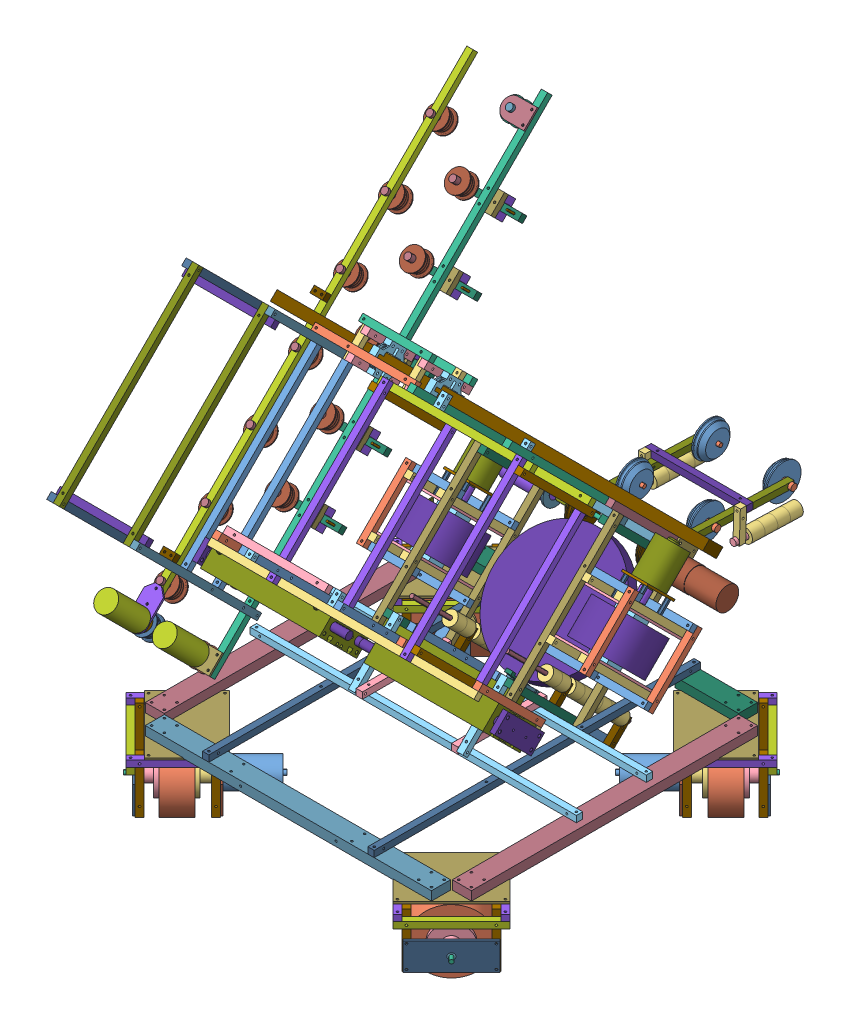
SolidWorks assembly R1, configuration ﾃﾞﾌｫﾙﾄ. Lengths in mm. (continued)
Components (placement in the parent): (continued)
- Copy of Shooter^R1-1: Copy of Shooter^R1 [ﾃﾞﾌｫﾙﾄ] at (-133.6161 -3.3981 632.9203) x (1 0 0) z (0 0.707107 0.707107) size (512.8 479.46 353.57) (virtual, flexible) (continued)
  - Copy of Copy (2) of Copy of Copy of Copy of Copy of Copy (2) of Copy of Copy (2) of 角材１^Copy of Shooter_R1-1: Copy of Copy (2) of Copy of Copy of Copy of Copy of Copy (2) of Copy of Copy (2) of 角材１^Copy of Shooter_R1 [ﾃﾞﾌｫﾙﾄ] at (170 10 140) x (0 0 -1) z (1 0 0) size (250 10 10) (virtual)
  - Part17^Copy of Shooter_R1-2: Part17^Copy of Shooter_R1 [ﾃﾞﾌｫﾙﾄ] at (35 45 -115) x (-0.307741 0.95147 0) z (0 0 1) size (6 6 270) (virtual)
  - Copy (2) of Copy of Copy of Copy of Copy of Copy (2) of Copy of Copy (2) of 角材１^Copy of Shooter_R1-5: Copy (2) of Copy of Copy of Copy of Copy of Copy (2) of Copy of Copy (2) of 角材１^Copy of Shooter_R1 [ﾃﾞﾌｫﾙﾄ] at (30 50 20) x (0 -1 0) z (0 0 1) size (50 10 10) (virtual)
  - Copy of Copy (2) of Copy of Copy of Copy of Copy of Copy (2) of Copy of Copy (2) of 角材１^Copy of Shooter_R1-2: Copy of Copy (2) of Copy of Copy of Copy of Copy of Copy (2) of Copy of Copy (2) of 角材１^Copy of Shooter_R1 [ﾃﾞﾌｫﾙﾄ] at (40 10 140) x (0 0 -1) z (1 0 0) size (250 10 10) (virtual)
  - Copy (3) of Copy of Copy of Copy of Copy of Copy (2) of Copy of Copy (2) of 角材１^Copy of Shooter_R1-1: Copy (3) of Copy of Copy of Copy of Copy of Copy (2) of Copy of Copy (2) of 角材１^Copy of Shooter_R1 [ﾃﾞﾌｫﾙﾄ] at (30 0 -100) size (160 10 10) (virtual)
  - Copy (2) of Copy of Copy of Copy of Copy of Copy (2) of Copy of Copy (2) of 角材１^Copy of Shooter_R1-6: Copy (2) of Copy of Copy of Copy of Copy of Copy (2) of Copy of Copy (2) of 角材１^Copy of Shooter_R1 [ﾃﾞﾌｫﾙﾄ] at (30 50 -110) x (0 -1 0) z (0 0 1) size (50 10 10) (virtual)
  - Copy (2) of Copy of Copy of Copy of Copy of Copy (2) of Copy of Copy (2) of 角材１^Copy of Shooter_R1-7: Copy (2) of Copy of Copy of Copy of Copy of Copy (2) of Copy of Copy (2) of 角材１^Copy of Shooter_R1 [ﾃﾞﾌｫﾙﾄ] at (180 50 -110) x (0 -1 0) z (0 0 1) size (50 10 10) (virtual)
  - Part20^Copy of Shooter_R1-1: Part20^Copy of Shooter_R1 [ﾃﾞﾌｫﾙﾄ] at (185 45 0) x (0 1 0) z (0 0 -1) size (21 21 20) (virtual)
  - Part20^Copy of Shooter_R1-2: Part20^Copy of Shooter_R1 [ﾃﾞﾌｫﾙﾄ] at (185 45 20) x (0 1 0) z (0 0 -1) size (21 21 20) (virtual)
  - Part20^Copy of Shooter_R1-3: Part20^Copy of Shooter_R1 [ﾃﾞﾌｫﾙﾄ] at (185 45 -80) x (0 1 0) z (0 0 -1) size (21 21 20) (virtual)
  - Part20^Copy of Shooter_R1-4: Part20^Copy of Shooter_R1 [ﾃﾞﾌｫﾙﾄ] at (185 45 -20) x (0 1 0) z (0 0 -1) size (21 21 20) (virtual)
  - Part20^Copy of Shooter_R1-5: Part20^Copy of Shooter_R1 [ﾃﾞﾌｫﾙﾄ] at (185 45 -60) x (0 1 0) z (0 0 -1) size (21 21 20) (virtual)
  - Part20^Copy of Shooter_R1-6: Part20^Copy of Shooter_R1 [ﾃﾞﾌｫﾙﾄ] at (185 45 -40) x (0.985931 0.167151 0) z (0 0 -1) size (21 21 20) (virtual)
  - Part20^Copy of Shooter_R1-7: Part20^Copy of Shooter_R1 [ﾃﾞﾌｫﾙﾄ] at (35 45 -20) x (0 1 0) z (0 0 -1) size (21 21 20) (virtual)
  - Part20^Copy of Shooter_R1-8: Part20^Copy of Shooter_R1 [ﾃﾞﾌｫﾙﾄ] at (35 45 20) x (0 1 0) z (0 0 -1) size (21 21 20) (virtual)
  - Part20^Copy of Shooter_R1-9: Part20^Copy of Shooter_R1 [ﾃﾞﾌｫﾙﾄ] at (35 45 -40) x (0 1 0) z (0 0 -1) size (21 21 20) (virtual)
  - Part20^Copy of Shooter_R1-10: Part20^Copy of Shooter_R1 [ﾃﾞﾌｫﾙﾄ] at (35 45 0) x (0 1 0) z (0 0 -1) size (21 21 20) (virtual)
  - Part20^Copy of Shooter_R1-11: Part20^Copy of Shooter_R1 [ﾃﾞﾌｫﾙﾄ] at (35 45 -60) x (0.234145 0.972202 0) z (0 0 -1) size (21 21 20) (virtual)
  - Part20^Copy of Shooter_R1-12: Part20^Copy of Shooter_R1 [ﾃﾞﾌｫﾙﾄ] at (35 45 -80) x (0 1 0) z (0 0 -1) size (21 21 20) (virtual)
  - Part20^Copy of Shooter_R1-21: Part20^Copy of Shooter_R1 [ﾃﾞﾌｫﾙﾄ] at (35 45 70) x (0 1 0) z (0 0 -1) size (21 21 20) (virtual)
  - Part20^Copy of Shooter_R1-22: Part20^Copy of Shooter_R1 [ﾃﾞﾌｫﾙﾄ] at (35 45 50) x (0 1 0) z (0 0 -1) size (21 21 20) (virtual)
  - Part20^Copy of Shooter_R1-23: Part20^Copy of Shooter_R1 [ﾃﾞﾌｫﾙﾄ] at (185 45 70) x (0.413014 0.910725 0) z (0 0 -1) size (21 21 20) (virtual)
  - Part20^Copy of Shooter_R1-24: Part20^Copy of Shooter_R1 [ﾃﾞﾌｫﾙﾄ] at (185 45 50) x (-0.320274 0.947325 0) z (0 0 -1) size (21 21 20) (virtual)
  - Copy of Copy of Copy of Copy (2) of Copy of Copy (2) of Copy of Copy (2) of 角材１^Copy of Shooter_R1-1: Copy of Copy of Copy of Copy (2) of Copy of Copy (2) of Copy of Copy (2) of 角材１^Copy of Shooter_R1 [ﾃﾞﾌｫﾙﾄ] at (190 16.9239 46.0051) x (0 -0.707107 0.707107) z (-1 0 0) size (140 10 10) (virtual)
  - Copy of Copy of Copy of Copy (2) of Copy of Copy (2) of Copy of Copy (2) of 角材１^Copy of Shooter_R1-2: Copy of Copy of Copy of Copy (2) of Copy of Copy (2) of Copy of Copy (2) of 角材１^Copy of Shooter_R1 [ﾃﾞﾌｫﾙﾄ] at (40 16.9239 46.0051) x (0 -0.707107 0.707107) z (-1 0 0) size (140 10 10) (virtual)
  - Copy (2) of Copy of Copy of Copy of Copy (2) of Copy of Copy (2) of 角材１^Copy of Shooter_R1-1: Copy (2) of Copy of Copy of Copy of Copy (2) of Copy of Copy (2) of 角材１^Copy of Shooter_R1 [ﾃﾞﾌｫﾙﾄ] at (190 20 150) x (0 -1 0) z (1 0 0) size (100 10 10) (virtual)
  - Copy (2) of Copy of Copy of Copy of Copy (2) of Copy of Copy (2) of 角材１^Copy of Shooter_R1-2: Copy (2) of Copy of Copy of Copy of Copy (2) of Copy of Copy (2) of 角材１^Copy of Shooter_R1 [ﾃﾞﾌｫﾙﾄ] at (20 20 150) x (0 -1 0) z (1 0 0) size (100 10 10) (virtual)
  - Copy of Part14^Copy of Shooter_R1-1: Copy of Part14^Copy of Shooter_R1 [ﾃﾞﾌｫﾙﾄ] at (45.4135 224.2591 -11.1142) x (0 0.083089 -0.996542) z (0 -0.996542 -0.083089) size (6 150 6) (virtual)
  - Copy of Copy of Copy (2) of Part36^Copy of Shooter_R1-1: Copy of Copy of Copy (2) of Part36^Copy of Shooter_R1 [ﾃﾞﾌｫﾙﾄ] at (36.0361 185.9032 -80.4602) x (0 0.839725 -0.543011) z (-1 0 0) size (16 16 18) (virtual)
  - Copy (2) of Copy of Part33^Copy of Shooter_R1-2: Copy (2) of Copy of Part33^Copy of Shooter_R1 [ﾃﾞﾌｫﾙﾄ] at (-597.1629 304.0265 -20) x (1 0 0) z (0 0 -1) size (90 32 32) (virtual)
  - Copy (2) of Copy (2) of Part36^Copy of Shooter_R1-2: Copy (2) of Copy (2) of Part36^Copy of Shooter_R1 [ﾃﾞﾌｫﾙﾄ] at (159 153.0001 -19.875) x (0 0.001736 0.999998) z (1 0 0) size (22 22 10) (virtual)
  - Copy of Copy of Part36^Copy of Shooter_R1-1: Copy of Copy of Part36^Copy of Shooter_R1 [ﾃﾞﾌｫﾙﾄ] at (180 153.1375 -24.4469) x (0 -0.061762 0.998091) z (1 0 0) size (22 22 10) (virtual)
  - Part22^Copy of Shooter_R1-1: Part22^Copy of Shooter_R1 [ﾃﾞﾌｫﾙﾄ] at (285 218 -20) x (0 0 1) z (0 -1 0) size (37 103 37) (virtual)
  - Part23^Copy of Shooter_R1-1: Part23^Copy of Shooter_R1 [ﾃﾞﾌｫﾙﾄ] at (203 240 -40) x (0 0 1) z (-1 0 0) size (40 52 3) (virtual)
  - Copy of Copy of Copy (2) of Copy of Copy of Copy of Copy of Copy (2) of Copy of Copy (2) of 角材１^Copy of Shooter_R1-1: Copy of Copy of Copy (2) of Copy of Copy of Copy of Copy of Copy (2) of Copy of Copy (2) of 角材１^Copy of Shooter_R1 [ﾃﾞﾌｫﾙﾄ] at (190 240 140) x (0 0 -1) z (1 0 0) size (180 10 10) (virtual)
  - Copy of Copy of Copy (2) of Copy of Copy of Copy of Copy of Copy (2) of Copy of Copy (2) of 角材１^Copy of Shooter_R1-2: Copy of Copy of Copy (2) of Copy of Copy of Copy of Copy of Copy (2) of Copy of Copy (2) of 角材１^Copy of Shooter_R1 [ﾃﾞﾌｫﾙﾄ] at (20 240 140) x (0 0 -1) z (1 0 0) size (180 10 10) (virtual)
  - Part24^Copy of Shooter_R1-1: Part24^Copy of Shooter_R1 [ﾃﾞﾌｫﾙﾄ] at (7 250 -40) x (0 0 1) z (1 0 0) size (40 45 3) (virtual)
  - Copy (4) of Copy of Copy of Copy of Copy of Copy (2) of Copy of Copy (2) of 角材１^Copy of Shooter_R1-2: Copy (4) of Copy of Copy of Copy of Copy of Copy (2) of Copy of Copy (2) of 角材１^Copy of Shooter_R1 [ﾃﾞﾌｫﾙﾄ] at (0 0 10) size (220 10 10) (virtual)
  - Copy (2) of Copy of Copy of Copy of Copy of Copy of Copy of Copy of Copy (2) of Copy of Copy (9) of Copy (2) of 角材１^Copy of Shooter_R1-3: Copy (2) of Copy of Copy of Copy of Copy of Copy of Copy of Copy of Copy (2) of Copy of Copy (9) of Copy (2) of 角材１^Copy of Shooter_R1 [ﾃﾞﾌｫﾙﾄ] at (50 218.3881 -5.6375) x (0 0.683966 -0.729514) z (-1 0 0) size (220 10 10) (virtual)
  - Copy (2) of Copy of Copy of Copy of Copy of Copy of Copy of Copy of Copy (2) of Copy of Copy (9) of Copy (2) of 角材１^Copy of Shooter_R1-4: Copy (2) of Copy of Copy of Copy of Copy of Copy of Copy of Copy of Copy (2) of Copy of Copy (9) of Copy (2) of 角材１^Copy of Shooter_R1 [ﾃﾞﾌｫﾙﾄ] at (180 218.3881 -5.6375) x (0 0.683966 -0.729514) z (-1 0 0) size (220 10 10) (virtual)
  - Copy of Copy of Copy of Copy (2) of Copy of Copy (2) of 角材１^Copy of Shooter_R1-1: Copy of Copy of Copy of Copy (2) of Copy of Copy (2) of 角材１^Copy of Shooter_R1 [ﾃﾞﾌｫﾙﾄ] at (190 324.8583 -104.5774) x (-1 0 0) z (0 -0.683966 0.729514) size (160 10 10) (virtual)
  - Part25^Copy of Shooter_R1-1: Part25^Copy of Shooter_R1 [ﾃﾞﾌｫﾙﾄ] at (170 225 -20) x (1 0 0) z (0 0.001736 0.999998) size (12 54 54) (virtual)
  - Part25^Copy of Shooter_R1-2: Part25^Copy of Shooter_R1 [ﾃﾞﾌｫﾙﾄ] at (50 225 -20) x (-1 0 0) z (0 0.001736 0.999998) size (12 54 54) (virtual)
  - Copy (2) of Copy (2) of Part36^Copy of Shooter_R1-3: Copy (2) of Copy (2) of Part36^Copy of Shooter_R1 [ﾃﾞﾌｫﾙﾄ] at (61 296.9999 -20.125) x (0 0.001736 0.999998) z (-1 0 0) size (22 22 10) (virtual)
  - Copy of Part25^Copy of Shooter_R1-3: Copy of Part25^Copy of Shooter_R1 [ﾃﾞﾌｫﾙﾄ] at (170 361.7931 -165.9028) x (1 0 0) z (0 0.037254 -0.999306) size (14 54 54) (virtual)
  - Part26^Copy of Shooter_R1-3: Part26^Copy of Shooter_R1 [ﾃﾞﾌｫﾙﾄ] at (185 361.7931 -165.9028) x (-1 0 0) z (0 0.008305 -0.999966) size (35 10 10) (virtual)
  - Part26^Copy of Shooter_R1-4: Part26^Copy of Shooter_R1 [ﾃﾞﾌｫﾙﾄ] at (35 361.7931 -165.9028) x (1 0 0) z (0 -0.001736 -0.999998) size (35 10 10) (virtual)
  - Copy of Part25^Copy of Shooter_R1-4: Copy of Part25^Copy of Shooter_R1 [ﾃﾞﾌｫﾙﾄ] at (50 361.7931 -165.9028) x (-1 0 0) z (0 -0.238788 -0.971072) size (14 54 54) (virtual)
  - Copy of Part25^Copy of Shooter_R1-5: Copy of Part25^Copy of Shooter_R1 [ﾃﾞﾌｫﾙﾄ] at (170 279.7173 -78.3611) x (1 0 0) z (0 0.999192 -0.040182) size (14 54 54) (virtual)
  - Part26^Copy of Shooter_R1-5: Part26^Copy of Shooter_R1 [ﾃﾞﾌｫﾙﾄ] at (185 279.7173 -78.3611) x (-1 0 0) z (0 -0.001736 -0.999998) size (35 10 10) (virtual)
  - Part26^Copy of Shooter_R1-6: Part26^Copy of Shooter_R1 [ﾃﾞﾌｫﾙﾄ] at (35 279.7173 -78.3611) x (1 0 0) z (0 -0.001736 -0.999998) size (35 10 10) (virtual)
  - Copy of Part25^Copy of Shooter_R1-6: Copy of Part25^Copy of Shooter_R1 [ﾃﾞﾌｫﾙﾄ] at (50 279.7173 -78.3611) x (-1 0 0) z (0 0.022457 -0.999748) size (14 54 54) (virtual)
  - Copy (3) of Copy of Copy of Copy of Copy (2) of Copy of Copy (2) of 角材１^Copy of Shooter_R1-1: Copy (3) of Copy of Copy of Copy of Copy (2) of Copy of Copy (2) of 角材１^Copy of Shooter_R1 [ﾃﾞﾌｫﾙﾄ] at (190 281.5429 -131.4805) x (0 0.729514 0.683966) z (0 -0.683966 0.729514) size (50 10 10) (virtual)
  - Copy (3) of Copy of Copy of Copy of Copy (2) of Copy of Copy (2) of 角材１^Copy of Shooter_R1-2: Copy (3) of Copy of Copy of Copy of Copy (2) of Copy of Copy (2) of 角材１^Copy of Shooter_R1 [ﾃﾞﾌｫﾙﾄ] at (40 281.5429 -131.4805) x (0 0.729514 0.683966) z (0 -0.683966 0.729514) size (50 10 10) (virtual)
  - Part20^Copy of Shooter_R1-25: Part20^Copy of Shooter_R1 [ﾃﾞﾌｫﾙﾄ] at (185 302.2896 -146.2985) x (0.035115 -0.729064 -0.683544) z (0 -0.683966 0.729514) size (21 21 20) (virtual)
  - Copy of Part26^Copy of Shooter_R1-1: Copy of Part26^Copy of Shooter_R1 [ﾃﾞﾌｫﾙﾄ] at (185 274.931 -117.118) x (0 0.683966 -0.729514) z (-0.990327 0.101225 0.094904) size (105 10 10) (virtual)
  - Part20^Copy of Shooter_R1-26: Part20^Copy of Shooter_R1 [ﾃﾞﾌｫﾙﾄ] at (185 315.9689 -160.8888) x (-0.121292 -0.724128 -0.678916) z (0 -0.683966 0.729514) size (21 21 20) (virtual)
  - Part20^Copy of Shooter_R1-27: Part20^Copy of Shooter_R1 [ﾃﾞﾌｫﾙﾄ] at (185 329.6482 -175.4791) x (0.035115 -0.729064 -0.683544) z (0 -0.683966 0.729514) size (21 21 20) (virtual)
  - Part20^Copy of Shooter_R1-28: Part20^Copy of Shooter_R1 [ﾃﾞﾌｫﾙﾄ] at (185 343.3275 -190.0694) x (0.035115 -0.729064 -0.683544) z (0 -0.683966 0.729514) size (21 21 20) (virtual)
  - Part20^Copy of Shooter_R1-29: Part20^Copy of Shooter_R1 [ﾃﾞﾌｫﾙﾄ] at (35 302.2896 -146.2985) x (0.035115 -0.729064 -0.683544) z (0 -0.683966 0.729514) size (21 21 20) (virtual)
  - Part20^Copy of Shooter_R1-30: Part20^Copy of Shooter_R1 [ﾃﾞﾌｫﾙﾄ] at (35 315.9689 -160.8888) x (-0.121292 -0.724128 -0.678916) z (0 -0.683966 0.729514) size (21 21 20) (virtual)
  - Copy of Part26^Copy of Shooter_R1-2: Copy of Part26^Copy of Shooter_R1 [ﾃﾞﾌｫﾙﾄ] at (35 274.931 -117.118) x (0 0.683966 -0.729514) z (-0.990327 0.101225 0.094904) size (105 10 10) (virtual)
  - Part20^Copy of Shooter_R1-31: Part20^Copy of Shooter_R1 [ﾃﾞﾌｫﾙﾄ] at (35 329.6482 -175.4791) x (0.035115 -0.729064 -0.683544) z (0 -0.683966 0.729514) size (21 21 20) (virtual)
  - Part20^Copy of Shooter_R1-32: Part20^Copy of Shooter_R1 [ﾃﾞﾌｫﾙﾄ] at (35 343.3275 -190.0694) x (0.035115 -0.729064 -0.683544) z (0 -0.683966 0.729514) size (21 21 20) (virtual)
  - Copy of Copy (4) of Copy of Copy of Copy of Copy (2) of Copy of Copy (2) of 角材１^Copy of Shooter_R1-1: Copy of Copy (4) of Copy of Copy of Copy of Copy (2) of Copy of Copy (2) of 角材１^Copy of Shooter_R1 [ﾃﾞﾌｫﾙﾄ] at (366.4 -75 137.9289) x (-1 0 0) z (0 -0.707107 -0.707107) size (512.8 10 10) (virtual)
  - Copy of Copy (4) of Copy of Copy of Copy of Copy (2) of Copy of Copy (2) of 角材１^Copy of Shooter_R1-2: Copy of Copy (4) of Copy of Copy of Copy of Copy (2) of Copy of Copy (2) of 角材１^Copy of Shooter_R1 [ﾃﾞﾌｫﾙﾄ] at (366.4 2.7817 60.1472) x (-1 0 0) z (0 -0.707107 -0.707107) size (512.8 10 10) (virtual)
- Copy of Assem3^R1-1: Copy of Assem3^R1 [ﾃﾞﾌｫﾙﾄ] at (-72.9957 96.2968 385.465) size (686.6 558.76 664.68) (virtual, flexible)
  - Assem5^Copy of Assem3_R1-1: Assem5^Copy of Assem3_R1 [ﾃﾞﾌｫﾙﾄ] at (161.552 -141.335 135.1971) x (1 0 0) z (0 0.000491 1) size (268.6 559.01 664.54) (virtual)
    - Copy of Copy of Copy of Copy of Copy of Copy of Copy of Part4^Assem5_Copy of Assem3_R1-1: Copy of Copy of Copy of Copy of Copy of Copy of Copy of Part4^Assem5_Copy of Assem3_R1 [ﾃﾞﾌｫﾙﾄ] at (-330.1724 90.9576 366.8614) x (1 0 0) z (0 0.70676 0.707454) size (10 750 10) (virtual)
    - Copy of Copy of Copy of Copy of Copy of Copy of Part4^Assem5_Copy of Assem3_R1-1: Copy of Copy of Copy of Copy of Copy of Copy of Part4^Assem5_Copy of Assem3_R1 [ﾃﾞﾌｫﾙﾄ] at (-430.1724 628.6154 -156.1339) x (-1 0 0) z (0 0.70676 0.707454) size (10 720 10) (virtual)
    - Copy of Copy of Copy of Part2^Assem5_Copy of Assem3_R1-1: Copy of Copy of Copy of Part2^Assem5_Copy of Assem3_R1 [ﾃﾞﾌｫﾙﾄ] at (-460.8277 161.547 253.7943) x (-1 0 0) z (0 -0.707454 0.70676) size (20 16 30) (virtual)
    - Copy of Copy of Copy of Copy of Copy of Copy (3) of Part3^Assem5_Copy of Assem3_R1-1: Copy of Copy of Copy of Copy of Copy of Copy (3) of Part3^Assem5_Copy of Assem3_R1 [ﾃﾞﾌｫﾙﾄ] at (-292.1724 156.3418 269.8784) x (0 0.70676 0.707454) z (0.847779 -0.375198 0.37483) size (27 4.5 4.5) (virtual)
    - Copy of Copy (2) of Copy of Copy (4) of Copy of Copy of Copy of Copy (2) of Copy of Copy (2) of 角材１^Assem5_Copy of Assem3_R1-1: Copy of Copy (2) of Copy of Copy (4) of Copy of Copy of Copy of Copy (2) of Copy of Copy (2) of 角材１^Assem5_Copy of Assem3_R1 [ﾃﾞﾌｫﾙﾄ] at (-440.1724 154.6215 317.3952) x (0 0.70676 0.707454) z (-1 0 0) size (260 10 10) (virtual)
    - Copy of Copy of Copy of Copy of Copy (2) of Copy of Copy (2) of Part11^Assem5_Copy of Assem3_R1-2: Copy of Copy of Copy of Copy of Copy (2) of Copy of Copy (2) of Part11^Assem5_Copy of Assem3_R1 [ﾃﾞﾌｫﾙﾄ] at (-435.1724 143.8683 327.8551) x (-0.731652 -0.482256 0.481783) z (-0.681679 0.51761 -0.517102) size (33.4 19.6 33.4) (virtual)
    - Copy of Copy of Copy of Copy of Part2^Assem5_Copy of Assem3_R1-1: Copy of Copy of Copy of Copy of Part2^Assem5_Copy of Assem3_R1 [ﾃﾞﾌｫﾙﾄ] at (-310.1724 182.9266 274.9826) x (1 0 0) z (0 -0.707454 0.70676) size (20 10 30) (virtual)
    - Copy of Copy of Copy of Copy (2) of Copy of Copy of Part5^Assem5_Copy of Assem3_R1-2: Copy of Copy of Copy of Copy (2) of Copy of Copy of Part5^Assem5_Copy of Assem3_R1 [ﾃﾞﾌｫﾙﾄ] at (-418.6839 156.0088 340.0168) x (1 -0.000283 0.000282) z (-0.0004 -0.707454 0.70676) size (10 45 10) (virtual)
    - Copy of Copy of Copy of Copy of Copy (4) of Copy of Copy of Copy of Copy (2) of Copy of Copy (2) of 角材１^Assem5_Copy of Assem3_R1-1: Copy of Copy of Copy of Copy of Copy (4) of Copy of Copy of Copy of Copy (2) of Copy of Copy (2) of 角材１^Assem5_Copy of Assem3_R1 [ﾃﾞﾌｫﾙﾄ] at (-320.1724 154.6284 303.253) x (0 0.70676 0.707454) z (1 0 0) size (270 10 10) (virtual)
    - Copy of Copy of Copy of Copy (3) of Copy of Copy of Copy (2) of Copy of Copy (2) of 角材１^Assem5_Copy of Assem3_R1-2: Copy of Copy of Copy of Copy (3) of Copy of Copy of Copy (2) of Copy of Copy (2) of 角材１^Assem5_Copy of Assem3_R1 [ﾃﾞﾌｫﾙﾄ] at (-282.1724 168.3602 274.8341) x (-1 0 0) z (0 -0.707454 0.70676) size (90 10 10) (virtual)
    - Copy of Copy of Copy of Copy of Copy (2) of Copy of Copy (2) of Part11^Assem5_Copy of Assem3_R1-17: Copy of Copy of Copy of Copy of Copy (2) of Copy of Copy (2) of Part11^Assem5_Copy of Assem3_R1 [ﾃﾞﾌｫﾙﾄ] at (-367.1724 164.823 278.3679) x (0.172855 -0.696805 0.696121) z (0.984947 0.122287 -0.122167) size (33.4 19.6 33.4) (virtual)
    - Copy of Copy of Copy of Copy (2) of Copy of Copy of Part5^Assem5_Copy of Assem3_R1-17: Copy of Copy of Copy of Copy (2) of Copy of Copy of Part5^Assem5_Copy of Assem3_R1 [ﾃﾞﾌｫﾙﾄ] at (-350.7089 153.4616 265.7105) x (0.998482 0.038963 -0.038925) z (-0.055075 0.70638 -0.705687) size (10 45 10) (virtual)
    - Copy of Copy of Copy of Copy (2) of Copy of Copy of Copy (2) of Copy of Copy (2) of 角材１^Assem5_Copy of Assem3_R1-1: Copy of Copy of Copy of Copy (2) of Copy of Copy of Copy (2) of Copy of Copy (2) of 角材１^Assem5_Copy of Assem3_R1 [ﾃﾞﾌｫﾙﾄ] at (-320.1724 550.622 275.1631) x (0 -0.707454 0.70676) z (-1 0 0) size (310 10 10) (virtual)
    - Copy of Copy (2) of Copy of Copy of Copy of Copy (2) of Copy of Copy (2) of 角材１^Assem5_Copy of Assem3_R1-1: Copy of Copy (2) of Copy of Copy of Copy of Copy (2) of Copy of Copy (2) of 角材１^Assem5_Copy of Assem3_R1 [ﾃﾞﾌｫﾙﾄ] at (-310.1724 338.3859 487.191) x (-1 0 0) z (0 -0.70676 -0.707454) size (140 10 10) (virtual)
    - Copy of Copy of Copy of Copy (2) of Copy of Copy of Copy (2) of Copy of Copy (2) of 角材１^Assem5_Copy of Assem3_R1-2: Copy of Copy of Copy of Copy (2) of Copy of Copy of Copy (2) of Copy of Copy (2) of 角材１^Assem5_Copy of Assem3_R1 [ﾃﾞﾌｫﾙﾄ] at (-430.1724 550.622 275.1631) x (0 -0.707454 0.70676) z (-1 0 0) size (310 10 10) (virtual)
    - Copy of Copy of Copy of Copy of Copy of Copy of Copy of Copy of Copy of 角材１^Assem5_Copy of Assem3_R1-1: Copy of Copy of Copy of Copy of Copy of Copy of Copy of Copy of Copy of 角材１^Assem5_Copy of Assem3_R1 [ﾃﾞﾌｫﾙﾄ] at (-430.1724 175.8381 310.3345) x (-1 0 0) z (0 0.70676 0.707454) size (20 10 10) (virtual)
    - Copy of Copy of Copy of Copy of Copy (2) of Copy of Copy of Copy (2) of Copy of Copy (2) of 角材１^Assem5_Copy of Assem3_R1-1: Copy of Copy of Copy of Copy of Copy (2) of Copy of Copy of Copy (2) of Copy of Copy (2) of 角材１^Assem5_Copy of Assem3_R1 [ﾃﾞﾌｫﾙﾄ] at (-350.1724 395.1418 105.3811) x (0 -0.707454 0.70676) z (-1 0 0) size (320 10 10) (virtual)
    - Copy of Copy (2) of Copy of Copy (4) of Copy of Copy of Copy of Copy (2) of Copy of Copy (2) of 角材１^Assem5_Copy of Assem3_R1-2: Copy of Copy (2) of Copy of Copy (4) of Copy of Copy of Copy of Copy (2) of Copy of Copy (2) of 角材１^Assem5_Copy of Assem3_R1 [ﾃﾞﾌｫﾙﾄ] at (-440.1724 366.8576 105.3672) x (0 0.70676 0.707454) z (-1 0 0) size (260 10 10) (virtual)
    - Copy of Copy (2) of Copy of Copy of Copy of Copy (2) of Copy of Copy (2) of 角材１^Assem5_Copy of Assem3_R1-2: Copy of Copy (2) of Copy of Copy of Copy of Copy (2) of Copy of Copy (2) of 角材１^Assem5_Copy of Assem3_R1 [ﾃﾞﾌｫﾙﾄ] at (-310.1724 536.473 289.2982) x (-1 0 0) z (0 -0.70676 -0.707454) size (140 10 10) (virtual)
    - Copy of Copy of Copy of Copy of Copy (4) of Copy of Copy of Copy of Copy (2) of Copy of Copy (2) of 角材１^Assem5_Copy of Assem3_R1-2: Copy of Copy of Copy of Copy of Copy (4) of Copy of Copy of Copy of Copy (2) of Copy of Copy (2) of 角材１^Assem5_Copy of Assem3_R1 [ﾃﾞﾌｫﾙﾄ] at (-320.1724 366.8645 91.2251) x (0 0.70676 0.707454) z (1 0 0) size (270 10 10) (virtual)
    - Copy of Copy of Copy of Copy of Copy (4) of Copy of Copy of Copy (2) of Copy of Copy (2) of 角材１^Assem5_Copy of Assem3_R1-1: Copy of Copy of Copy of Copy of Copy (4) of Copy of Copy of Copy (2) of Copy of Copy (2) of 角材１^Assem5_Copy of Assem3_R1 [ﾃﾞﾌｫﾙﾄ] at (-200.1724 388.0742 98.3066) x (-1 0 0) z (0 0.70676 0.707454) size (160 10 10) (virtual)
    - Copy of Copy of Copy of Copy of Copy of Copy (2) of Copy of Copy of Copy of Copy (2) of Copy of Copy (2) of 角材１^Assem5_Copy of Assem3_R1-1: Copy of Copy of Copy of Copy of Copy of Copy (2) of Copy of Copy of Copy of Copy (2) of Copy of Copy (2) of 角材１^Assem5_Copy of Assem3_R1 [ﾃﾞﾌｫﾙﾄ] at (-310.1724 380.9928 119.5163) x (0 0.707454 -0.70676) z (1 0 0) size (55 10 10) (virtual)
    - Copy of Copy of Copy of Copy (2) of Copy of Copy of Copy of Copy (2) of Copy of Copy (2) of 角材１^Assem5_Copy of Assem3_R1-1: Copy of Copy of Copy of Copy (2) of Copy of Copy of Copy of Copy (2) of Copy of Copy (2) of 角材１^Assem5_Copy of Assem3_R1 [ﾃﾞﾌｫﾙﾄ] at (-290.1724 476.4365 151.3829) x (0 -0.70676 -0.707454) z (-1 0 0) size (100 10 10) (virtual)
    - Copy of Copy of Copy of Copy of Copy of Copy of NHK_r1_guide.STL^Assem5_Copy of Assem3_R1-1: Copy of Copy of Copy of Copy of Copy of Copy of NHK_r1_guide.STL^Assem5_Copy of Assem3_R1 [ﾃﾞﾌｫﾙﾄ] at (-280.1724 419.8958 94.7867) x (0 -0.707454 0.70676) z (-1 0 0) size (45 60 10) (virtual)
    - Copy of Copy of Copy of Copy (4) of Copy of Copy of Copy (2) of Copy of Copy (2) of 角材１^Assem5_Copy of Assem3_R1-1: Copy of Copy of Copy of Copy (4) of Copy of Copy of Copy (2) of Copy of Copy (2) of 角材１^Assem5_Copy of Assem3_R1 [ﾃﾞﾌｫﾙﾄ] at (-200.1724 476.4435 137.2408) x (-1 0 0) z (0 0.70676 0.707454) size (110 10 10) (virtual)
    - Copy of Copy of Copy of Copy (2) of Copy of Copy of Copy of Copy (2) of Copy of Copy (2) of 角材１^Assem5_Copy of Assem3_R1-2: Copy of Copy of Copy of Copy (2) of Copy of Copy of Copy of Copy (2) of Copy of Copy (2) of 角材１^Assem5_Copy of Assem3_R1 [ﾃﾞﾌｫﾙﾄ] at (-290.1724 451.6757 176.1195) x (0 -0.70676 -0.707454) z (-1 0 0) size (100 10 10) (virtual)
    - Copy of Copy of Copy of Copy of Copy of Copy (2) of Copy of Copy of Copy of Copy (2) of Copy of Copy (2) of 角材１^Assem5_Copy of Assem3_R1-2: Copy of Copy of Copy of Copy of Copy of Copy (2) of Copy of Copy of Copy of Copy (2) of Copy of Copy (2) of 角材１^Assem5_Copy of Assem3_R1 [ﾃﾞﾌｫﾙﾄ] at (-310.1724 430.4659 169.0381) x (0 0.707454 -0.70676) z (1 0 0) size (55 10 10) (virtual)
    - Copy of Copy of Copy of Copy of Copy (4) of Copy of Copy of Copy (2) of Copy of Copy (2) of 角材１^Assem5_Copy of Assem3_R1-2: Copy of Copy of Copy of Copy of Copy (4) of Copy of Copy of Copy (2) of Copy of Copy (2) of 角材１^Assem5_Copy of Assem3_R1 [ﾃﾞﾌｫﾙﾄ] at (-200.1724 451.6826 161.9774) x (-1 0 0) z (0 0.70676 0.707454) size (160 10 10) (virtual)
    - Copy of Copy of Copy of Copy of Copy of Copy (2) of Copy of Copy of Copy of Copy (2) of Copy of Copy (2) of 角材１^Assem5_Copy of Assem3_R1-3: Copy of Copy of Copy of Copy of Copy of Copy (2) of Copy of Copy of Copy of Copy (2) of Copy of Copy (2) of 角材１^Assem5_Copy of Assem3_R1 [ﾃﾞﾌｫﾙﾄ] at (-220.1724 430.4659 169.0381) x (0 0.707454 -0.70676) z (1 0 0) size (55 10 10) (virtual)
    - Copy of Copy of Copy of Copy (2) of Copy of Copy of Copy of Copy (2) of Copy of Copy (2) of 角材１^Assem5_Copy of Assem3_R1-3: Copy of Copy of Copy of Copy (2) of Copy of Copy of Copy of Copy (2) of Copy of Copy (2) of 角材１^Assem5_Copy of Assem3_R1 [ﾃﾞﾌｫﾙﾄ] at (-200.1724 451.6757 176.1195) x (0 -0.70676 -0.707454) z (-1 0 0) size (100 10 10) (virtual)
    - Copy of Copy of Copy of Copy (4) of Copy of Copy of Copy (2) of Copy of Copy (2) of 角材１^Assem5_Copy of Assem3_R1-2: Copy of Copy of Copy of Copy (4) of Copy of Copy of Copy (2) of Copy of Copy (2) of 角材１^Assem5_Copy of Assem3_R1 [ﾃﾞﾌｫﾙﾄ] at (-200.1724 412.8351 73.57) x (-1 0 0) z (0 0.70676 0.707454) size (110 10 10) (virtual)
    - Copy of Copy of Copy of Copy of Copy of Copy (2) of Copy of Copy of Copy of Copy (2) of Copy of Copy (2) of 角材１^Assem5_Copy of Assem3_R1-4: Copy of Copy of Copy of Copy of Copy of Copy (2) of Copy of Copy of Copy of Copy (2) of Copy of Copy (2) of 角材１^Assem5_Copy of Assem3_R1 [ﾃﾞﾌｫﾙﾄ] at (-220.1724 380.9928 119.5163) x (0 0.707454 -0.70676) z (1 0 0) size (55 10 10) (virtual)
    - Copy of Copy of Copy of Copy (2) of Copy of Copy of Copy of Copy (2) of Copy of Copy (2) of 角材１^Assem5_Copy of Assem3_R1-4: Copy of Copy of Copy of Copy (2) of Copy of Copy of Copy of Copy (2) of Copy of Copy (2) of 角材１^Assem5_Copy of Assem3_R1 [ﾃﾞﾌｫﾙﾄ] at (-200.1724 476.4365 151.3829) x (0 -0.70676 -0.707454) z (-1 0 0) size (100 10 10) (virtual)
    - Copy of Copy of Copy of Copy of Copy of Copy of NHK_r1_guide.STL^Assem5_Copy of Assem3_R1-2: Copy of Copy of Copy of Copy of Copy of Copy of NHK_r1_guide.STL^Assem5_Copy of Assem3_R1 [ﾃﾞﾌｫﾙﾄ] at (-190.1724 419.8958 94.7867) x (0 -0.707454 0.70676) z (-1 0 0) size (45 60 10) (virtual)
    - Copy of Copy of Copy of Copy of Copy of Copy of Copy of Copy of Copy of 角材１^Assem5_Copy of Assem3_R1-3: Copy of Copy of Copy of Copy of Copy of Copy of Copy of Copy of Copy of 角材１^Assem5_Copy of Assem3_R1 [ﾃﾞﾌｫﾙﾄ] at (-430.1724 412.8351 73.57) x (-1 0 0) z (0 0.70676 0.707454) size (20 10 10) (virtual)
    - Copy of Copy of Copy of roller_R1^Assem5_Copy of Assem3_R1-1: Copy of Copy of Copy of roller_R1^Assem5_Copy of Assem3_R1 [ﾃﾞﾌｫﾙﾄ] at (53.8339 52.095 142.792) x (0.212331 0 0.977198) z (0 1 0) (virtual)
    - Copy of Copy of Copy of Copy of Copy (2) of Copy of Copy of Copy (2) of Copy of Copy (2) of 角材１^Assem5_Copy of Assem3_R1-2: Copy of Copy of Copy of Copy of Copy (2) of Copy of Copy of Copy (2) of Copy of Copy (2) of 角材１^Assem5_Copy of Assem3_R1 [ﾃﾞﾌｫﾙﾄ] at (-350.1724 444.615 154.9029) x (0 -0.707454 0.70676) z (-1 0 0) size (320 10 10) (virtual)
    - Copy of Copy of Copy of Copy (2) of Copy of Copy of Part5^Assem5_Copy of Assem3_R1-5: Copy of Copy of Copy of Copy (2) of Copy of Copy of Part5^Assem5_Copy of Assem3_R1 [ﾃﾞﾌｫﾙﾄ] at (-418.6839 297.4995 198.6648) x (1 -0.000283 0.000282) z (-0.0004 -0.707454 0.70676) size (10 45 10) (virtual)
    - Copy of Copy of Copy of Copy (2) of Copy of Copy of Part5^Assem5_Copy of Assem3_R1-6: Copy of Copy of Copy of Copy (2) of Copy of Copy of Part5^Assem5_Copy of Assem3_R1 [ﾃﾞﾌｫﾙﾄ] at (-418.6839 368.2449 127.9889) x (1 -0.000283 0.000282) z (-0.0004 -0.707454 0.70676) size (10 45 10) (virtual)
    - Copy of Copy of Copy of Copy (2) of Copy of Copy of Part5^Assem5_Copy of Assem3_R1-7: Copy of Copy of Copy of Copy (2) of Copy of Copy of Part5^Assem5_Copy of Assem3_R1 [ﾃﾞﾌｫﾙﾄ] at (-418.6839 438.9903 57.3129) x (1 -0.000283 0.000282) z (-0.0004 -0.707454 0.70676) size (10 45 10) (virtual)
    - Copy of Copy of Copy of Copy (2) of Copy of Copy of Part5^Assem5_Copy of Assem3_R1-8: Copy of Copy of Copy of Copy (2) of Copy of Copy of Part5^Assem5_Copy of Assem3_R1 [ﾃﾞﾌｫﾙﾄ] at (-418.6839 509.7356 -13.3631) x (1 -0.000283 0.000282) z (-0.0004 -0.707454 0.70676) size (10 45 10) (virtual)
    - Copy of Copy of Copy of Copy of Copy (2) of Copy of Copy (2) of Part11^Assem5_Copy of Assem3_R1-5: Copy of Copy of Copy of Copy of Copy (2) of Copy of Copy (2) of Part11^Assem5_Copy of Assem3_R1 [ﾃﾞﾌｫﾙﾄ] at (-435.1724 285.359 186.5031) x (-0.731652 -0.482256 0.481783) z (-0.681679 0.51761 -0.517102) size (33.4 19.6 33.4) (virtual)
    - Copy of Copy of Copy of Copy of Copy (2) of Copy of Copy (2) of Part11^Assem5_Copy of Assem3_R1-6: Copy of Copy of Copy of Copy of Copy (2) of Copy of Copy (2) of Part11^Assem5_Copy of Assem3_R1 [ﾃﾞﾌｫﾙﾄ] at (-435.1724 356.1044 115.8271) x (-0.731652 -0.482256 0.481783) z (-0.681679 0.51761 -0.517102) size (33.4 19.6 33.4) (virtual)
    - Copy of Copy of Copy of Copy of Copy (2) of Copy of Copy (2) of Part11^Assem5_Copy of Assem3_R1-7: Copy of Copy of Copy of Copy of Copy (2) of Copy of Copy (2) of Part11^Assem5_Copy of Assem3_R1 [ﾃﾞﾌｫﾙﾄ] at (-435.1724 426.8498 45.1512) x (-0.731652 -0.482256 0.481783) z (-0.681679 0.51761 -0.517102) size (33.4 19.6 33.4) (virtual)
    - Copy of Copy of Copy of Copy of Copy (2) of Copy of Copy (2) of Part11^Assem5_Copy of Assem3_R1-8: Copy of Copy of Copy of Copy of Copy (2) of Copy of Copy (2) of Part11^Assem5_Copy of Assem3_R1 [ﾃﾞﾌｫﾙﾄ] at (-435.1724 497.5951 -25.5248) x (-0.731652 -0.482256 0.481783) z (-0.681679 0.51761 -0.517102) size (33.4 19.6 33.4) (virtual)
    - Copy of Copy of Copy of Copy (2) of Copy of Copy of Part5^Assem5_Copy of Assem3_R1-18: Copy of Copy of Copy of Copy (2) of Copy of Copy of Part5^Assem5_Copy of Assem3_R1 [ﾃﾞﾌｫﾙﾄ] at (-350.7089 224.207 195.0345) x (0.998482 0.038963 -0.038925) z (-0.055075 0.70638 -0.705687) size (10 45 10) (virtual)
    - Copy of Copy of Copy of Copy (2) of Copy of Copy of Part5^Assem5_Copy of Assem3_R1-19: Copy of Copy of Copy of Copy (2) of Copy of Copy of Part5^Assem5_Copy of Assem3_R1 [ﾃﾞﾌｫﾙﾄ] at (-350.7089 294.9523 124.3585) x (0.998482 0.038963 -0.038925) z (-0.055075 0.70638 -0.705687) size (10 45 10) (virtual)
    - Copy of Copy of Copy of Copy (2) of Copy of Copy of Part5^Assem5_Copy of Assem3_R1-20: Copy of Copy of Copy of Copy (2) of Copy of Copy of Part5^Assem5_Copy of Assem3_R1 [ﾃﾞﾌｫﾙﾄ] at (-350.7089 365.6977 53.6825) x (0.998482 0.038963 -0.038925) z (-0.055075 0.70638 -0.705687) size (10 45 10) (virtual)
    - Copy of Copy of Copy of Copy (2) of Copy of Copy of Part5^Assem5_Copy of Assem3_R1-21: Copy of Copy of Copy of Copy (2) of Copy of Copy of Part5^Assem5_Copy of Assem3_R1 [ﾃﾞﾌｫﾙﾄ] at (-350.7089 436.4431 -16.9934) x (0.998482 0.038963 -0.038925) z (-0.055075 0.70638 -0.705687) size (10 45 10) (virtual)
    - Copy of Copy of Copy of Copy (2) of Copy of Copy of Part5^Assem5_Copy of Assem3_R1-22: Copy of Copy of Copy of Copy (2) of Copy of Copy of Part5^Assem5_Copy of Assem3_R1 [ﾃﾞﾌｫﾙﾄ] at (-350.7089 507.1884 -87.6694) x (0.998482 0.038963 -0.038925) z (-0.055075 0.70638 -0.705687) size (10 45 10) (virtual)
    - Copy of Copy of Copy of Copy of Copy (2) of Copy of Copy (2) of Part11^Assem5_Copy of Assem3_R1-18: Copy of Copy of Copy of Copy of Copy (2) of Copy of Copy (2) of Part11^Assem5_Copy of Assem3_R1 [ﾃﾞﾌｫﾙﾄ] at (-367.1724 235.5683 207.6919) x (0.172855 -0.696805 0.696121) z (0.984947 0.122287 -0.122167) size (33.4 19.6 33.4) (virtual)
    - Copy of Copy of Copy of Copy of Copy (2) of Copy of Copy (2) of Part11^Assem5_Copy of Assem3_R1-19: Copy of Copy of Copy of Copy of Copy (2) of Copy of Copy (2) of Part11^Assem5_Copy of Assem3_R1 [ﾃﾞﾌｫﾙﾄ] at (-367.1724 306.3137 137.0159) x (0.172855 -0.696805 0.696121) z (0.984947 0.122287 -0.122167) size (33.4 19.6 33.4) (virtual)
    - Copy of Copy of Copy of Copy of Copy (2) of Copy of Copy (2) of Part11^Assem5_Copy of Assem3_R1-20: Copy of Copy of Copy of Copy of Copy (2) of Copy of Copy (2) of Part11^Assem5_Copy of Assem3_R1 [ﾃﾞﾌｫﾙﾄ] at (-367.1724 377.0591 66.3399) x (0.172855 -0.696805 0.696121) z (0.984947 0.122287 -0.122167) size (33.4 19.6 33.4) (virtual)
    - Copy of Copy of Copy of Copy of Copy (2) of Copy of Copy (2) of Part11^Assem5_Copy of Assem3_R1-21: Copy of Copy of Copy of Copy of Copy (2) of Copy of Copy (2) of Part11^Assem5_Copy of Assem3_R1 [ﾃﾞﾌｫﾙﾄ] at (-367.1724 447.8044 -4.336) x (0.172855 -0.696805 0.696121) z (0.984947 0.122287 -0.122167) size (33.4 19.6 33.4) (virtual)
    - Copy of Copy of Copy of Copy of Copy (2) of Copy of Copy (2) of Part11^Assem5_Copy of Assem3_R1-22: Copy of Copy of Copy of Copy of Copy (2) of Copy of Copy (2) of Part11^Assem5_Copy of Assem3_R1 [ﾃﾞﾌｫﾙﾄ] at (-367.1724 518.5498 -75.012) x (0.172855 -0.696805 0.696121) z (0.984947 0.122287 -0.122167) size (33.4 19.6 33.4) (virtual)
    - Copy of Copy of Copy of Copy of Part2^Assem5_Copy of Assem3_R1-2: Copy of Copy of Copy of Copy of Part2^Assem5_Copy of Assem3_R1 [ﾃﾞﾌｫﾙﾄ] at (-310.1724 253.6719 204.3067) x (1 0 0) z (0 -0.707454 0.70676) size (20 10 30) (virtual)
    - Copy of Copy of Copy of Copy of Part2^Assem5_Copy of Assem3_R1-3: Copy of Copy of Copy of Copy of Part2^Assem5_Copy of Assem3_R1 [ﾃﾞﾌｫﾙﾄ] at (-310.1724 324.4173 133.6307) x (1 0 0) z (0 -0.707454 0.70676) size (20 10 30) (virtual)
    - Copy of Copy of Copy of Copy of Part2^Assem5_Copy of Assem3_R1-4: Copy of Copy of Copy of Copy of Part2^Assem5_Copy of Assem3_R1 [ﾃﾞﾌｫﾙﾄ] at (-310.1724 395.1626 62.9547) x (1 0 0) z (0 -0.707454 0.70676) size (20 10 30) (virtual)
    - Copy of Copy of Copy of Copy of Part2^Assem5_Copy of Assem3_R1-5: Copy of Copy of Copy of Copy of Part2^Assem5_Copy of Assem3_R1 [ﾃﾞﾌｫﾙﾄ] at (-310.1724 465.908 -7.7213) x (1 0 0) z (0 -0.707454 0.70676) size (20 10 30) (virtual)
    - Copy of Copy of Copy of Copy of Part2^Assem5_Copy of Assem3_R1-6: Copy of Copy of Copy of Copy of Part2^Assem5_Copy of Assem3_R1 [ﾃﾞﾌｫﾙﾄ] at (-310.1724 536.6534 -78.3972) x (1 0 0) z (0 -0.707454 0.70676) size (20 10 30) (virtual)
    - Copy of Copy of Copy of Part2^Assem5_Copy of Assem3_R1-2: Copy of Copy of Copy of Part2^Assem5_Copy of Assem3_R1 [ﾃﾞﾌｫﾙﾄ] at (-460.8277 232.2923 183.1183) x (-1 0 0) z (0 -0.707454 0.70676) size (20 16 30) (virtual)
    - Copy of Copy of Copy of Part2^Assem5_Copy of Assem3_R1-3: Copy of Copy of Copy of Part2^Assem5_Copy of Assem3_R1 [ﾃﾞﾌｫﾙﾄ] at (-460.8277 303.0377 112.4423) x (-1 0 0) z (0 -0.707454 0.70676) size (20 16 30) (virtual)
    - Copy of Copy of Copy of Part2^Assem5_Copy of Assem3_R1-4: Copy of Copy of Copy of Part2^Assem5_Copy of Assem3_R1 [ﾃﾞﾌｫﾙﾄ] at (-460.8277 373.7831 41.7664) x (-1 0 0) z (0 -0.707454 0.70676) size (20 16 30) (virtual)
    - Copy of Copy of Copy of Part2^Assem5_Copy of Assem3_R1-5: Copy of Copy of Copy of Part2^Assem5_Copy of Assem3_R1 [ﾃﾞﾌｫﾙﾄ] at (-460.8277 444.5284 -28.9096) x (-1 0 0) z (0 -0.707454 0.70676) size (20 16 30) (virtual)
    - Copy of Copy of Copy of Part2^Assem5_Copy of Assem3_R1-6: Copy of Copy of Copy of Part2^Assem5_Copy of Assem3_R1 [ﾃﾞﾌｫﾙﾄ] at (-460.8277 515.2738 -99.5856) x (-1 0 0) z (0 -0.707454 0.70676) size (20 16 30) (virtual)
    - Copy of Copy of Copy of Copy of Copy of Copy (3) of Part3^Assem5_Copy of Assem3_R1-2: Copy of Copy of Copy of Copy of Copy of Copy (3) of Part3^Assem5_Copy of Assem3_R1 [ﾃﾞﾌｫﾙﾄ] at (-292.1724 227.0872 199.2024) x (0 0.70676 0.707454) z (0.847779 -0.375198 0.37483) size (27 4.5 4.5) (virtual)
    - Copy of Copy of Copy of Copy of Copy of Copy (3) of Part3^Assem5_Copy of Assem3_R1-3: Copy of Copy of Copy of Copy of Copy of Copy (3) of Part3^Assem5_Copy of Assem3_R1 [ﾃﾞﾌｫﾙﾄ] at (-292.1724 297.8326 128.5265) x (0 0.70676 0.707454) z (0.847779 -0.375198 0.37483) size (27 4.5 4.5) (virtual)
    - Copy of Copy of Copy of Copy of Copy of Copy (3) of Part3^Assem5_Copy of Assem3_R1-4: Copy of Copy of Copy of Copy of Copy of Copy (3) of Part3^Assem5_Copy of Assem3_R1 [ﾃﾞﾌｫﾙﾄ] at (-292.1724 368.5779 57.8505) x (0 0.70676 0.707454) z (0.847779 -0.375198 0.37483) size (27 4.5 4.5) (virtual)
    - Copy of Copy of Copy of Copy of Copy of Copy (3) of Part3^Assem5_Copy of Assem3_R1-5: Copy of Copy of Copy of Copy of Copy of Copy (3) of Part3^Assem5_Copy of Assem3_R1 [ﾃﾞﾌｫﾙﾄ] at (-292.1724 439.3233 -12.8255) x (0 0.70676 0.707454) z (0.847779 -0.375198 0.37483) size (27 4.5 4.5) (virtual)
    - Copy of Copy of Copy of Copy of Copy of Copy (3) of Part3^Assem5_Copy of Assem3_R1-6: Copy of Copy of Copy of Copy of Copy of Copy (3) of Part3^Assem5_Copy of Assem3_R1 [ﾃﾞﾌｫﾙﾄ] at (-292.1724 510.0687 -83.5014) x (0 0.70676 0.707454) z (0.847779 -0.375198 0.37483) size (27 4.5 4.5) (virtual)
    - Copy of Copy of Copy of Copy (3) of Copy of Copy of Copy (2) of Copy of Copy (2) of 角材１^Assem5_Copy of Assem3_R1-3: Copy of Copy of Copy of Copy (3) of Copy of Copy of Copy (2) of Copy of Copy (2) of 角材１^Assem5_Copy of Assem3_R1 [ﾃﾞﾌｫﾙﾄ] at (-282.1724 239.1056 204.1581) x (-1 0 0) z (0 -0.707454 0.70676) size (90 10 10) (virtual)
    - Copy of Copy of Copy of Copy (3) of Copy of Copy of Copy (2) of Copy of Copy (2) of 角材１^Assem5_Copy of Assem3_R1-4: Copy of Copy of Copy of Copy (3) of Copy of Copy of Copy (2) of Copy of Copy (2) of 角材１^Assem5_Copy of Assem3_R1 [ﾃﾞﾌｫﾙﾄ] at (-282.1724 309.851 133.4821) x (-1 0 0) z (0 -0.707454 0.70676) size (90 10 10) (virtual)
